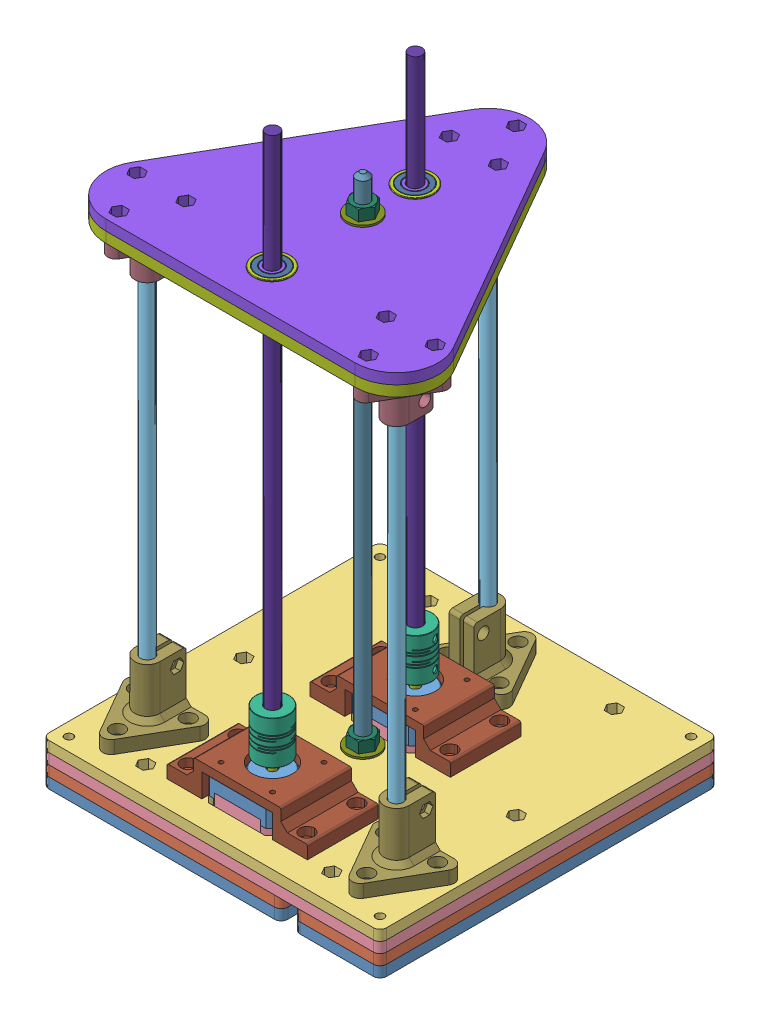
SolidWorks assembly 02_00_Assy_z_axis_V1, configuration Défaut. Lengths in mm.
Overall size (203.2 380.91 203.2).
110 component instances, 54 part files, 69 mates.
Components (placement in the parent):
- 02_01_Assy_base_z_axis_V1-1: 02_01_Assy_base_z_axis_V1 [Défaut] at (-233.6469 0 294.9138) size (203.2 25.4 203.2)
  - 02_03_plaque_fond_base-1: 02_03_plaque_fond_base [Défaut] at (80.101 0 119.7934) size (203.2 6.35 203.2)
  - 02_05_deuxieme_niveau_base-1: 02_05_deuxieme_niveau_base [Défaut] at (80.101 6.35 119.7934) x (-1 0 0) z (0 0 -1) size (203.2 6.35 203.2)
  - 02_06_troixieme_niveau_base-1: 02_06_troixieme_niveau_base [Défaut] at (80.101 19.05 119.7934) x (-1 0 0) z (0 0 -1) size (203.2 6.35 203.2)
  - 02_012_deuxieme_v2_niveau_base-1: 02_012_deuxieme_v2_niveau_base [Défaut] at (80.101 12.7 119.7934) x (-1 0 0) z (0 0 -1) size (203.2 6.35 203.2)
- Stainless_Steel_Rod_8_290-1: Stainless_Steel_Rod_8_290 [1274T471] at (-228.5459 151.35 479.7071) x (0.927753 0 -0.373195) z (0 -1 0) size (8 8 290)
- Stainless_Steel_Rod_8_290-2: Stainless_Steel_Rod_8_290 [1274T471] at (-78.5444 151.35 479.7063) x (-0.988682 0 -0.150024) z (0 -1 0) size (8 8 290)
- Stainless_Steel_Rod_8_290-3: Stainless_Steel_Rod_8_290 [1274T471] at (-153.5459 151.35 349.7071) x (-0.878649 0 -0.477467) z (0 1 0) size (8 8 290)
- NEMA17_Coupler-1: NEMA17_Coupler [Default] at (-153.3959 48.5 479.5571) x (-0.967472 0 -0.252977) z (0.252977 0 -0.967472) size (26.77 26 23.11)
- 02_09_support_trois_rods_haut-1: 02_09_support_trois_rods_haut [Défaut] at (-153.5451 290 414.7071) x (-1 0 0.000011) z (-0.000011 0 -1) size (200 6.35 180)
- 02_10_support_haut-1: 02_10_support_haut [Défaut] at (-153.5451 296.35 414.7071) x (-1 0 0.000011) z (-0.000011 0 -1) size (200 6.35 180)
- 608-2RS Skate Board Ball Bearing.step-2: 608-2RS Skate Board Ball Bearing.step [Défaut] at (-153.5444 299.85 479.7071) x (0 -1 0) z (0 0 1) size (7 22 22)
  - Ball 001.step-1: Ball 001.step [Défaut] at origin size (4 4 4)
  - Ball 002.step-1: Ball 002.step [Défaut] x (1 0 0) z (0 0.781831 0.62349) size (4 4 4)
  - Ball 003.step-1: Ball 003.step [Défaut] x (1 0 0) z (0 0.974928 -0.222521) size (4 4 4)
  - Ball 004.step-1: Ball 004.step [Défaut] x (1 0 0) z (0 0.433884 -0.900969) size (4 4 4)
  - Ball 005.step-1: Ball 005.step [Défaut] x (1 0 0) z (0 -0.433884 -0.900969) size (4 4 4)
  - Ball 006.step-1: Ball 006.step [Défaut] x (1 0 0) z (0 -0.974928 -0.222521) size (4 4 4)
  - Ball 007.step-1: Ball 007.step [Défaut] x (1 0 0) z (0 -0.781831 0.62349) size (4 4 4)
  - Cage 001.step-1: Cage 001.step [Défaut] x (1 0 0) z (0 1 0) size (2.12 17 16.8)
  - Cage 002.step-1: Cage 002.step [Défaut] x (-1 0 0) z (0 0 -1) size (2.12 16.8 17)
  - Rivet 002.step-1: Rivet 002.step [Défaut] x (1 0 0) z (0 -0.781831 0.62349) size (0.42 0.6 0.6)
  - Rivet 003.step-1: Rivet 003.step [Défaut] x (1 0 0) z (0 -0.974928 -0.222521) size (0.42 0.6 0.6)
  - Rivet 001.step-1: Rivet 001.step [Défaut] x (1 0 0) z (0 -0.433884 0.900969) size (0.42 0.6 0.6)
  - Rivet 004.step-1: Rivet 004.step [Défaut] x (1 0 0) z (0 -0.433884 -0.900969) size (0.42 0.6 0.6)
  - Rivet 005.step-1: Rivet 005.step [Défaut] x (1 0 0) z (0 0.433884 -0.900969) size (0.42 0.6 0.6)
  - Rivet 006.step-1: Rivet 006.step [Défaut] x (1 0 0) z (0 0.974928 -0.222521) size (0.42 0.6 0.6)
  - Rivet 007.step-1: Rivet 007.step [Défaut] x (1 0 0) z (0 0.781831 0.62349) size (0.42 0.6 0.6)
  - Outer Ring001.step-1: Outer Ring001.step [Défaut] at origin size (7 22 22)
  - Inner Ring001.step-1: Inner Ring001.step [Défaut] at origin size (7 12 12)
  - Seal 001.step-1: Seal 001.step [Défaut] at origin size (0.6 19 19)
  - Seal 002.step-1: Seal 002.step [Défaut] x (-1 0 0) z (0 0 -1) size (0.6 19 19)
- 02_11_support_moteur-1: 02_11_support_moteur [Défaut] at (-153.3959 39.5 479.5571) size (84.5 19.1 42.5)
- 02_13_support_rodes_8mm_base-1: 02_13_support_rodes_8mm_base [Défaut] at (-78.5444 25.4 479.7063) x (-1 0 0) z (0 0 -1) size (47.68 37.8 42.63)
- 02_13_support_rodes_8mm_base-2: 02_13_support_rodes_8mm_base [Défaut] at (-228.5459 25.4 479.7071) x (-1 0 0) z (0 0 -1) size (47.68 37.8 42.63)
- 02_13_support_rodes_8mm_base-3: 02_13_support_rodes_8mm_base [Défaut] at (-153.5459 25.4 349.7071) size (47.68 37.8 42.63)
- 02_14_support_rodes_8mm_haut-1: 02_14_support_rodes_8mm_haut [Défaut] at (-78.5444 290 479.7063) x (1 0 -0.000011) z (-0.000011 0 -1) size (42.68 27.8 38.3)
- 02_14_support_rodes_8mm_haut-2: 02_14_support_rodes_8mm_haut [Défaut] at (-228.5459 290 479.7071) x (1 0 -0.000011) z (-0.000011 0 -1) size (42.68 27.8 38.3)
- 02_14_support_rodes_8mm_haut-3: 02_14_support_rodes_8mm_haut [Défaut] at (-153.5459 290 349.7071) x (-1 0 0.000011) z (0.000011 0 1) size (42.68 27.8 38.3)
- Lead Screw_M12-1: Lead Screw_M12 [97048A742] at (-153.5459 162.5 425.0321) x (-0.414721 0 0.909949) z (0 -1 0) size (7.9 7.9 325)
- 95462A510_Medium-Strength Steel Hex Nut-2: 95462A510_Medium-Strength Steel Hex Nut [95462A510] at (-153.5459 307.1656 425.0321) x (0.86602 0 -0.50001) z (0 1 0) size (12.7 14.66 6.75)
- 516_washer-1: 516_washer [90107A030] at (-153.5459 302.7 425.0321) size (19.05 1.09 19.05)
- 516_washer-2: 516_washer [90107A030] at (-153.5459 25.4 425.0321) size (19.05 1.09 19.05)
- T8_lead_screw_300mm-1: T8_lead_screw_300mm [1274T471] at (-153.3959 223.9115 479.5571) x (0.654232 0 0.756294) z (0 1 0) size (8 8 300)
- 02_11_support_moteur-2: 02_11_support_moteur [Défaut] at (-153.3959 39.5 393.5571) size (84.5 19.1 42.5)
- 95462A510_Medium-Strength Steel Hex Nut-4: 95462A510_Medium-Strength Steel Hex Nut [95462A510] at (-153.5459 29.8656 425.0321) x (0.866025 0 -0.5) z (0 1 0) size (12.7 14.66 6.75)
- 608-2RS Skate Board Ball Bearing.step-3: 608-2RS Skate Board Ball Bearing.step [Défaut] at (-153.5454 299.85 393.7071) x (0 -1 0) z (0.672808 0 0.739817) size (7 22 22)
  - Ball 001.step-1: Ball 001.step [Défaut] at origin size (4 4 4)
  - Ball 002.step-1: Ball 002.step [Défaut] x (1 0 0) z (0 0.781831 0.62349) size (4 4 4)
  - Ball 003.step-1: Ball 003.step [Défaut] x (1 0 0) z (0 0.974928 -0.222521) size (4 4 4)
  - Ball 004.step-1: Ball 004.step [Défaut] x (1 0 0) z (0 0.433884 -0.900969) size (4 4 4)
  - Ball 005.step-1: Ball 005.step [Défaut] x (1 0 0) z (0 -0.433884 -0.900969) size (4 4 4)
  - Ball 006.step-1: Ball 006.step [Défaut] x (1 0 0) z (0 -0.974928 -0.222521) size (4 4 4)
  - Ball 007.step-1: Ball 007.step [Défaut] x (1 0 0) z (0 -0.781831 0.62349) size (4 4 4)
  - Cage 001.step-1: Cage 001.step [Défaut] x (1 0 0) z (0 1 0) size (2.12 17 16.8)
  - Cage 002.step-1: Cage 002.step [Défaut] x (-1 0 0) z (0 0 -1) size (2.12 16.8 17)
  - Rivet 002.step-1: Rivet 002.step [Défaut] x (1 0 0) z (0 -0.781831 0.62349) size (0.42 0.6 0.6)
  - Rivet 003.step-1: Rivet 003.step [Défaut] x (1 0 0) z (0 -0.974928 -0.222521) size (0.42 0.6 0.6)
  - Rivet 001.step-1: Rivet 001.step [Défaut] x (1 0 0) z (0 -0.433884 0.900969) size (0.42 0.6 0.6)
  - Rivet 004.step-1: Rivet 004.step [Défaut] x (1 0 0) z (0 -0.433884 -0.900969) size (0.42 0.6 0.6)
  - Rivet 005.step-1: Rivet 005.step [Défaut] x (1 0 0) z (0 0.433884 -0.900969) size (0.42 0.6 0.6)
  - Rivet 006.step-1: Rivet 006.step [Défaut] x (1 0 0) z (0 0.974928 -0.222521) size (0.42 0.6 0.6)
  - Rivet 007.step-1: Rivet 007.step [Défaut] x (1 0 0) z (0 0.781831 0.62349) size (0.42 0.6 0.6)
  - Outer Ring001.step-1: Outer Ring001.step [Défaut] at origin size (7 22 22)
  - Inner Ring001.step-1: Inner Ring001.step [Défaut] at origin size (7 12 12)
  - Seal 001.step-1: Seal 001.step [Défaut] at origin size (0.6 19 19)
  - Seal 002.step-1: Seal 002.step [Défaut] x (-1 0 0) z (0 0 -1) size (0.6 19 19)
- NEMA17_Coupler-2: NEMA17_Coupler [Default] at (-153.3959 48.5 393.5571) x (-0.262561 0 -0.964915) z (0.964915 0 -0.262561) size (26.77 26 23.11)
- T8_lead_screw_300mm-2: T8_lead_screw_300mm [1274T471] at (-153.3959 222 393.5571) x (0.996676 0 0.081473) z (0 -1 0) size (8 8 300)
- 95462A510_Medium-Strength Steel Hex Nut-5: 95462A510_Medium-Strength Steel Hex Nut [95462A510] at (-153.5459 3.3734 425.0321) x (0.866025 0 -0.5) z (0 -1 0) size (12.7 14.66 6.75)
- NEMA17 x 33.step-1: NEMA17 x 33.step [Défaut] at (-153.3959 39.5 393.5571) x (0 0 1) z (1 0 0) size (42 70.5 60)
  - Copper-2of4.step-1: Copper-2of4.step [Défaut] at (0 28 0) x (0 1 0) z (0 0 1) size (2.77 3.05 24)
  - Frontplate.step-1: Frontplate.step [Défaut] at (0 10.5 0) size (42 12.5 42)
  - Backplate.step-1: Backplate.step [Défaut] at (0 33 0) size (42 10.5 42)
  - Connenctor.step-1: Connenctor.step [Défaut] at (0 24.5 22) size (7 7 7)
  - Housing.step-1: Housing.step [Défaut] at (0 7.5 0) size (42 32 42)
  - Bearing dummy.step-1: Bearing dummy.step [Défaut] at (0 4 0) size (22 7 22)
  - Bearing dummy 01.step-1: Bearing dummy 01.step [Défaut] at (0 28 0) size (22 7 22)
  - Core.step-1: Core.step [Défaut] at origin size (30 70.5 30)
  - M3x25-Screw.step-1: M3x25-Screw.step [Défaut] at (15.5 30.6 15.5) x (1 0 0) z (0 1 0) size (5.5 5.5 27)
  - M3x25-Screw004.step-1: M3x25-Screw004.step [Défaut] at (-15.5 30.6 15.5) x (1 0 0) z (0 1 0) size (5.5 5.5 27)
  - M3x25-Screw005.step-1: M3x25-Screw005.step [Défaut] at (-15.5 30.6 -15.5) x (1 0 0) z (0 1 0) size (5.5 5.5 27)
  - M3x25-Screw006.step-1: M3x25-Screw006.step [Défaut] at (15.5 30.6 -15.5) x (1 0 0) z (0 1 0) size (5.5 5.5 27)
  - Cable-1of4.step-1: Cable-1of4.step [Défaut] at (0 28 0) size (3.44 3.69 21)
  - Copper-1of4.step-1: Copper-1of4.step [Défaut] at (0 28 0) size (2.77 3.05 24)
  - Cable-2of4.step-1: Cable-2of4.step [Défaut] at (0 28 0) x (0 1 0) z (0 0 1) size (3.44 3.69 21)
  - Copper-4of4.step-1: Copper-4of4.step [Défaut] at (0 28 0) x (0 -1 0) z (0 0 1) size (2.77 3.05 24)
  - Cable-3of4.step-1: Cable-3of4.step [Défaut] at (0 28 0) x (-1 0 0) z (0 0 1) size (3.44 3.69 21)
  - Copper-3of4.step-1: Copper-3of4.step [Défaut] at (0 28 0) x (-1 0 0) z (0 0 1) size (2.77 3.05 24)
  - Cable-4of4.step-1: Cable-4of4.step [Défaut] at (0 28 0) x (0 -1 0) z (0 0 1) size (3.44 3.69 21)
- NEMA17 x 33.step-2: NEMA17 x 33.step [Défaut] at (-153.3959 39.5 479.5571) x (0 0 1) z (1 0 0) size (42 70.5 60)
  - Copper-2of4.step-1: Copper-2of4.step [Défaut] at (0 28 0) x (0 1 0) z (0 0 1) size (2.77 3.05 24)
  - Frontplate.step-1: Frontplate.step [Défaut] at (0 10.5 0) size (42 12.5 42)
  - Backplate.step-1: Backplate.step [Défaut] at (0 33 0) size (42 10.5 42)
  - Connenctor.step-1: Connenctor.step [Défaut] at (0 24.5 22) size (7 7 7)
  - Housing.step-1: Housing.step [Défaut] at (0 7.5 0) size (42 32 42)
  - Bearing dummy.step-1: Bearing dummy.step [Défaut] at (0 4 0) size (22 7 22)
  - Bearing dummy 01.step-1: Bearing dummy 01.step [Défaut] at (0 28 0) size (22 7 22)
  - Core.step-1: Core.step [Défaut] at origin size (30 70.5 30)
  - M3x25-Screw.step-1: M3x25-Screw.step [Défaut] at (15.5 30.6 15.5) x (1 0 0) z (0 1 0) size (5.5 5.5 27)
  - M3x25-Screw004.step-1: M3x25-Screw004.step [Défaut] at (-15.5 30.6 15.5) x (1 0 0) z (0 1 0) size (5.5 5.5 27)
  - M3x25-Screw005.step-1: M3x25-Screw005.step [Défaut] at (-15.5 30.6 -15.5) x (1 0 0) z (0 1 0) size (5.5 5.5 27)
  - M3x25-Screw006.step-1: M3x25-Screw006.step [Défaut] at (15.5 30.6 -15.5) x (1 0 0) z (0 1 0) size (5.5 5.5 27)
  - Cable-1of4.step-1: Cable-1of4.step [Défaut] at (0 28 0) size (3.44 3.69 21)
  - Copper-1of4.step-1: Copper-1of4.step [Défaut] at (0 28 0) size (2.77 3.05 24)
  - Cable-2of4.step-1: Cable-2of4.step [Défaut] at (0 28 0) x (0 1 0) z (0 0 1) size (3.44 3.69 21)
  - Copper-4of4.step-1: Copper-4of4.step [Défaut] at (0 28 0) x (0 -1 0) z (0 0 1) size (2.77 3.05 24)
  - Cable-3of4.step-1: Cable-3of4.step [Défaut] at (0 28 0) x (-1 0 0) z (0 0 1) size (3.44 3.69 21)
  - Copper-3of4.step-1: Copper-3of4.step [Défaut] at (0 28 0) x (-1 0 0) z (0 0 1) size (2.77 3.05 24)
  - Cable-4of4.step-1: Cable-4of4.step [Défaut] at (0 28 0) x (0 -1 0) z (0 0 1) size (3.44 3.69 21)
Mates (geometry in assembly coordinates):
- Coïncidente1: coincident anti-aligned: plane of 02_01_Assy_base_z_axis_V1-1/02_03_plaque_fond_base-1 through (-153.5459 0 414.7071) normal (0 -1 0)
- Coïncidente4: coincident anti-aligned: plane of 02_01_Assy_base_z_axis_V1-1/02_03_plaque_fond_base-1 through (-153.5459 6.35 414.7071) normal (0 1 0); plane of Stainless_Steel_Rod_8_290-1 through (-228.5459 6.35 479.7071) normal (0 -1 0)
- Coïncidente5: coincident anti-aligned: plane of 02_01_Assy_base_z_axis_V1-1/02_03_plaque_fond_base-1 through (-153.5459 6.35 414.7071) normal (0 1 0); plane of Stainless_Steel_Rod_8_290-2 through (-78.5444 6.35 479.7063) normal (0 -1 0)
- Coïncidente6: coincident anti-aligned: plane of 02_01_Assy_base_z_axis_V1-1/02_03_plaque_fond_base-1 through (-153.5459 6.35 414.7071) normal (0 1 0); plane of Stainless_Steel_Rod_8_290-3 through (-153.5459 6.35 349.7071) normal (0 -1 0)
- Coïncidente29: coincident aligned: plane of Stainless_Steel_Rod_8_290-1 through (-228.5459 296.35 479.7071) normal (0 1 0); plane of 02_09_support_trois_rods_haut-1 through (-78.5444 296.35 479.7063) normal (0 1 0)
- Coaxiale20: concentric aligned: cylinder of Stainless_Steel_Rod_8_290-3 through (-153.5459 296.35 349.7071) axis (0 -1 0) radius 4; cylinder of 02_09_support_trois_rods_haut-1 through (-153.5459 296.35 349.7071) axis (0 -1 0) radius 3.925
- Coaxiale21: concentric anti-aligned: cylinder of Stainless_Steel_Rod_8_290-2 through (-78.5444 6.35 479.7063) axis (0 1 0) radius 4; cylinder of 02_09_support_trois_rods_haut-1 through (-78.5444 296.35 479.7063) axis (0 -1 0) radius 3.925
- Coïncidente30: coincident anti-aligned: plane of 02_09_support_trois_rods_haut-1 through (-78.5444 296.35 479.7063) normal (0 1 0); plane of 02_10_support_haut-1 through (-78.5444 296.35 479.7063) normal (0 -1 0)
- Coaxiale22: concentric aligned: cylinder of 02_09_support_trois_rods_haut-1 through (-153.5444 296.35 479.7071) axis (0 -1 0) radius 5.7; cylinder of 02_10_support_haut-1 through (-153.5444 302.7 479.7071) axis (0 -1 0) radius 11
- Coïncidente31: coincident aligned: plane of 02_09_support_trois_rods_haut-1 through (-56.8899 296.35 467.213) normal (0.86618 0 -0.499732); plane of 02_10_support_haut-1 through (-56.8899 302.7 467.213) normal (0.86618 0 -0.499732)
- Coïncidente32: coincident anti-aligned: plane of 02_09_support_trois_rods_haut-1 through (-78.5444 296.35 479.7063) normal (0 1 0); plane of 608-2RS Skate Board Ball Bearing.step-2/Inner Ring001.step-1 through (-153.5444 296.35 479.7071) normal (0 -1 0)
- Coaxiale23: concentric anti-aligned: cylinder of 02_09_support_trois_rods_haut-1 through (-153.5444 296.35 479.7071) axis (0 -1 0) radius 5.7; cylinder of 608-2RS Skate Board Ball Bearing.step-2/Inner Ring001.step-1 through (-153.5444 296.35 479.7071) axis (0 1 0) radius 4
- Coaxiale26: concentric aligned: cylinder of Stainless_Steel_Rod_8_290-2 through (-78.5444 6.35 479.7063) axis (0 1 0) radius 4; cylinder of 02_13_support_rodes_8mm_base-1 through (-78.5444 25.4 479.7063) axis (0 1 0) radius 4.075
- Coïncidente36: coincident anti-aligned: plane of 02_01_Assy_base_z_axis_V1-1/02_06_troixieme_niveau_base-1 through (-153.5459 25.4 414.7071) normal (0 1 0); plane of 02_13_support_rodes_8mm_base-1 through (-78.5444 25.4 479.7063) normal (0 -1 0)
- Coaxiale27: concentric anti-aligned: cylinder of Stainless_Steel_Rod_8_290-3 through (-153.5459 296.35 349.7071) axis (0 -1 0) radius 4; cylinder of 02_13_support_rodes_8mm_base-3 through (-153.5459 25.4 349.7071) axis (0 1 0) radius 4.075
- Coïncidente38: coincident anti-aligned: plane of 02_01_Assy_base_z_axis_V1-1/02_06_troixieme_niveau_base-1 through (-153.5459 25.4 414.7071) normal (0 1 0); plane of 02_13_support_rodes_8mm_base-3 through (-153.5459 25.4 349.7071) normal (0 -1 0)
- Parallèle3: parallel anti-aligned: plane of 02_01_Assy_base_z_axis_V1-1/02_06_troixieme_niveau_base-1 through (-51.9459 25.4 516.3071) normal (0 0 1); plane of 02_13_support_rodes_8mm_base-1 through (-51.0444 33.2 463.8292) normal (0 0 -1)
- Coïncidente41: coincident anti-aligned: plane of 02_01_Assy_base_z_axis_V1-1/02_06_troixieme_niveau_base-1 through (-153.5459 25.4 414.7071) normal (0 1 0); plane of 02_13_support_rodes_8mm_base-2 through (-228.5459 25.4 479.7071) normal (0 -1 0)
- Coaxiale28: concentric aligned: cylinder of Stainless_Steel_Rod_8_290-1 through (-228.5459 6.35 479.7071) axis (0 1 0) radius 4; cylinder of 02_13_support_rodes_8mm_base-2 through (-228.5459 25.4 479.7071) axis (0 1 0) radius 4.075
- Parallèle4: parallel anti-aligned: plane of 02_01_Assy_base_z_axis_V1-1/02_06_troixieme_niveau_base-1 through (-51.9459 25.4 516.3071) normal (0 0 1); plane of 02_13_support_rodes_8mm_base-2 through (-201.0459 33.2 463.83) normal (0 0 -1)
- Coïncidente46: coincident anti-aligned: plane of 02_09_support_trois_rods_haut-1 through (-78.5444 290 479.7063) normal (0 -1 0); plane of 02_14_support_rodes_8mm_haut-2 through (-228.5459 290 479.7071) normal (0 1 0)
- Coaxiale30: concentric anti-aligned: cylinder of Stainless_Steel_Rod_8_290-1 through (-228.5459 6.35 479.7071) axis (0 1 0) radius 4; cylinder of 02_14_support_rodes_8mm_haut-2 through (-228.5459 290 479.7071) axis (0 -1 0) radius 4.075
- Parallèle5: parallel anti-aligned: plane of 02_09_support_trois_rods_haut-1 through (-78.5441 296.35 504.7063) normal (0.000011 0 1); plane of 02_14_support_rodes_8mm_haut-2 through (-253.546 282.2 465.2737) normal (-0.000011 0 -1)
- Coïncidente48: coincident anti-aligned: plane of 02_09_support_trois_rods_haut-1 through (-78.5444 290 479.7063) normal (0 -1 0); plane of 02_14_support_rodes_8mm_haut-1 through (-78.5444 290 479.7063) normal (0 1 0)
- Coaxiale31: concentric anti-aligned: cylinder of 02_14_support_rodes_8mm_haut-1 through (-78.5444 290 479.7063) axis (0 -1 0) radius 4.075; cylinder of Stainless_Steel_Rod_8_290-2 through (-78.5444 6.35 479.7063) axis (0 1 0) radius 4
- Parallèle7: parallel anti-aligned: plane of 02_09_support_trois_rods_haut-1 through (-78.5441 296.35 504.7063) normal (0.000011 0 1); plane of 02_14_support_rodes_8mm_haut-1 through (-103.5446 282.2 465.2728) normal (-0.000011 0 -1)
- Coïncidente51: coincident anti-aligned: plane of 02_09_support_trois_rods_haut-1 through (-78.5444 290 479.7063) normal (0 -1 0); plane of 02_14_support_rodes_8mm_haut-3 through (-153.5459 290 349.7071) normal (0 1 0)
- Coaxiale32: concentric aligned: cylinder of Stainless_Steel_Rod_8_290-3 through (-153.5459 296.35 349.7071) axis (0 -1 0) radius 4; cylinder of 02_14_support_rodes_8mm_haut-3 through (-153.5459 290 349.7071) axis (0 -1 0) radius 4.075
- Coaxiale34: concentric anti-aligned: cylinder of 02_10_support_haut-1 through (-153.5459 296.35 425.0321) axis (0 1 0) radius 4; cylinder of Lead Screw_M12-1 through (-153.5459 0 425.0321) axis (0 -1 0) radius 3.95
- Coïncidente52: coincident aligned: plane of 02_01_Assy_base_z_axis_V1-1/02_03_plaque_fond_base-1 through (-153.5459 0 414.7071) normal (0 -1 0); plane of Lead Screw_M12-1 through (-157.1402 0 423.394) normal (0 -1 0)
- Coaxiale38: concentric anti-aligned: cylinder of 02_01_Assy_base_z_axis_V1-1/02_06_troixieme_niveau_base-1 through (-153.5459 19.05 349.7071) axis (0 1 0) radius 3.925; cylinder of Stainless_Steel_Rod_8_290-3 through (-153.5459 296.35 349.7071) axis (0 -1 0) radius 4
- Parallèle13: parallel anti-aligned: plane of 02_01_Assy_base_z_axis_V1-1/02_03_plaque_fond_base-1 through (-255.1459 6.35 313.1071) normal (0 0 -1); plane of 02_13_support_rodes_8mm_base-3 through (-181.0459 33.2 365.5843) normal (0 0 1)
- Parallèle14: parallel aligned: plane of 02_09_support_trois_rods_haut-1 through (-78.5441 296.35 504.7063) normal (0.000011 0 1); plane of 02_14_support_rodes_8mm_haut-3 through (-128.5457 282.2 364.1406) normal (0.000011 0 1)
- Coaxiale43: concentric aligned: cylinder of 02_01_Assy_base_z_axis_V1-1/02_06_troixieme_niveau_base-1 through (-228.5459 19.05 479.7071) axis (0 1 0) radius 3.925; cylinder of Stainless_Steel_Rod_8_290-1 through (-228.5459 6.35 479.7071) axis (0 1 0) radius 4
- Parallèle15: parallel anti-aligned: plane of 02_01_Assy_base_z_axis_V1-1/02_06_troixieme_niveau_base-1 through (-51.9459 25.4 516.3071) normal (0 0 1); plane of 02_13_support_rodes_8mm_base-2 through (-201.0459 33.2 463.83) normal (0 0 -1)
- Coaxiale48: concentric aligned: cylinder of Lead Screw_M12-1 through (-153.5459 0 425.0321) axis (0 -1 0) radius 3.95; cylinder of 95462A510_Medium-Strength Steel Hex Nut-2 through (-153.5459 310.5391 425.0321) axis (0 -1 0) radius 3.9688
- Coaxiale49: concentric anti-aligned: cylinder of Lead Screw_M12-1 through (-153.5459 0 425.0321) axis (0 -1 0) radius 3.95; cylinder of 516_washer-1 through (-153.5459 302.7 425.0321) axis (0 1 0) radius 4.3688
- Coïncidente69: coincident anti-aligned: plane of 02_10_support_haut-1 through (-78.5444 302.7 479.7063) normal (0 1 0); plane of 516_washer-1 through (-153.5459 302.7 425.0321) normal (0 -1 0)
- Coïncidente70: coincident anti-aligned: plane of 95462A510_Medium-Strength Steel Hex Nut-2 through (-160.8782 303.7922 425.0322) normal (0 -1 0); plane of 516_washer-1 through (-153.5459 303.7922 425.0321) normal (0 1 0)
- Parallèle19: parallel aligned: plane of 02_10_support_haut-1 through (-78.5441 302.7 504.7063) normal (0.000011 0 1); plane of 95462A510_Medium-Strength Steel Hex Nut-2 through (-157.212 310.5391 431.3822) normal (0.000011 0 1)
- Coïncidente72: coincident anti-aligned: plane of 02_01_Assy_base_z_axis_V1-1/02_06_troixieme_niveau_base-1 through (-153.5459 25.4 414.7071) normal (0 1 0); plane of 516_washer-2 through (-153.5459 25.4 425.0321) normal (0 -1 0)
- Coaxiale53: concentric aligned: cylinder of NEMA17_Coupler-1 through (-153.3959 48.5 479.5571) axis (0 -1 0) radius 4.025; cylinder of T8_lead_screw_300mm-1 through (-153.3959 373.9115 479.5571) axis (0 -1 0) radius 4
- Coaxiale58: concentric aligned: cylinder of 02_01_Assy_base_z_axis_V1-1/02_06_troixieme_niveau_base-1 through (-153.5459 19.05 425.0321) axis (0 1 0) radius 4; cylinder of 516_washer-2 through (-153.5459 25.4 425.0321) axis (0 1 0) radius 4.3688
- Coïncidente84: coincident: plane of 02_11_support_moteur-1 through (-179.6459 39.5 479.5571) normal (-1 0 0); plane of 02_11_support_moteur-2 through (-179.6459 61.288 393.5571) normal (-1 0 0)
- Coaxiale61: concentric anti-aligned: cylinder of Lead Screw_M12-1 through (-153.5459 0 425.0321) axis (0 -1 0) radius 3.95; circle of 95462A510_Medium-Strength Steel Hex Nut-4
- Coïncidente89: coincident anti-aligned: plane of 516_washer-2 through (-153.5459 26.4922 425.0321) normal (0 1 0); plane of 95462A510_Medium-Strength Steel Hex Nut-4 through (-160.8782 26.4922 425.0321) normal (0 -1 0)
- Parallèle25: parallel aligned: plane of 02_01_Assy_base_z_axis_V1-1/02_06_troixieme_niveau_base-1 through (-51.9459 25.4 516.3071) normal (0 0 1); plane of 95462A510_Medium-Strength Steel Hex Nut-4 through (-157.2121 33.2391 431.3821) normal (0 0 1)
- Coaxiale62: concentric anti-aligned: cylinder of 02_10_support_haut-1 through (-153.5454 296.35 393.7071) axis (0 1 0) radius 11; cylinder of 608-2RS Skate Board Ball Bearing.step-3/Outer Ring001.step-1 through (-153.5454 303.35 393.7071) axis (0 -1 0) radius 11
- Coïncidente91: coincident anti-aligned: plane of 02_09_support_trois_rods_haut-1 through (-78.5444 296.35 479.7063) normal (0 1 0); plane of 608-2RS Skate Board Ball Bearing.step-3/Outer Ring001.step-1 through (-153.5454 296.35 393.7071) normal (0 -1 0)
- Coaxiale64: concentric anti-aligned: cylinder of NEMA17_Coupler-2 through (-153.3959 48.5 393.5571) axis (0 -1 0) radius 4.025; cylinder of T8_lead_screw_300mm-2 through (-153.3959 72 393.5571) axis (0 1 0) radius 4
- Coaxiale65: concentric anti-aligned: cylinder of Lead Screw_M12-1 through (-153.5459 0 425.0321) axis (0 -1 0) radius 3.95; cylinder of 95462A510_Medium-Strength Steel Hex Nut-5 through (-153.5459 0 425.0321) axis (0 1 0) radius 3.9688
- Coaxiale66: concentric anti-aligned: cylinder of 02_01_Assy_base_z_axis_V1-1/02_012_deuxieme_v2_niveau_base-1 through (-153.5459 12.7 425.0321) axis (0 1 0) radius 4; cylinder of Lead Screw_M12-1 through (-153.5459 0 425.0321) axis (0 -1 0) radius 3.95
- Parallèle26: parallel aligned: plane of 02_01_Assy_base_z_axis_V1-1/02_03_plaque_fond_base-1 through (-157.1976 0 418.7071) normal (0.866025 0 0.5); plane of 95462A510_Medium-Strength Steel Hex Nut-5 through (-146.2135 0 425.0321) normal (0.866025 0 0.5)
- Coïncidente95: coincident aligned: plane of 02_01_Assy_base_z_axis_V1-1/02_03_plaque_fond_base-1 through (-153.5459 0 414.7071) normal (0 -1 0); plane of 95462A510_Medium-Strength Steel Hex Nut-5 through (-157.2121 0 431.3821) normal (0 -1 0)
- Coïncidente97: coincident aligned: plane of 02_01_Assy_base_z_axis_V1-1/02_03_plaque_fond_base-1 through (-153.5459 0 414.7071) normal (0 -1 0); plane of NEMA17 x 33.step-2/Housing.step-1 through (-153.3959 0 479.5571) normal (0 -1 0)
- Coïncidente98: coincident aligned: plane of 02_01_Assy_base_z_axis_V1-1/02_03_plaque_fond_base-1 through (-153.5459 0 414.7071) normal (0 -1 0); plane of NEMA17 x 33.step-1/Housing.step-1 through (-153.3959 0 393.5571) normal (0 -1 0)
- Coïncidente99: coincident anti-aligned: plane of 02_01_Assy_base_z_axis_V1-1/02_03_plaque_fond_base-1 through (-132.3959 0 462.7291) normal (-1 0 0); plane of NEMA17 x 33.step-2/Housing.step-1 through (-132.3959 32 465.718) normal (1 0 0)
- Coïncidente100: coincident anti-aligned: plane of 02_01_Assy_base_z_axis_V1-1/02_06_troixieme_niveau_base-1 through (-136.5678 19.05 458.5571) normal (0 0 1); plane of NEMA17 x 33.step-2/Frontplate.step-1 through (-136.4253 29 458.5571) normal (0 0 -1)
- Coïncidente101: coincident anti-aligned: plane of 02_01_Assy_base_z_axis_V1-1/02_06_troixieme_niveau_base-1 through (-132.3959 19.05 376.7291) normal (-1 0 0); plane of NEMA17 x 33.step-1/Frontplate.step-1 through (-132.3959 29 410.5277) normal (1 0 0)
- Coïncidente102: coincident anti-aligned: plane of 02_01_Assy_base_z_axis_V1-1/02_06_troixieme_niveau_base-1 through (-170.5239 19.05 372.5571) normal (0 0 1); plane of NEMA17 x 33.step-1/Frontplate.step-1 through (-136.4253 29 372.5571) normal (0 0 -1)
- Coïncidente103: coincident anti-aligned: plane of NEMA17_Coupler-1 through (-156.0758 48.5 478.8564) normal (0 -1 0); plane of NEMA17 x 33.step-2/Core.step-1 through (-151.1459 48.5 479.5571) normal (0 1 0)
- Coaxiale69: concentric aligned: circle of NEMA17_Coupler-1; cylinder of NEMA17 x 33.step-2/Core.step-1 through (-153.3959 63.2 479.5571) axis (0 -1 0) radius 2.5
- Coïncidente104: coincident anti-aligned: plane of NEMA17_Coupler-2 through (-154.1232 48.5 390.8843) normal (0 -1 0); plane of NEMA17 x 33.step-1/Core.step-1 through (-151.1459 48.5 393.5571) normal (0 1 0)
- Coaxiale70: concentric aligned: circle of NEMA17_Coupler-2; cylinder of NEMA17 x 33.step-1/Core.step-1 through (-153.3959 63.2 393.5571) axis (0 -1 0) radius 2.5
- Coaxiale73: concentric anti-aligned: cylinder of 02_11_support_moteur-1 through (-168.8959 39.5 495.0571) axis (0 1 0) radius 1.325; cylinder of NEMA17 x 33.step-2/Frontplate.step-1 through (-168.8959 29 495.0571) axis (0 -1 0) radius 1.23
- Coaxiale74: concentric anti-aligned: cylinder of 02_11_support_moteur-1 through (-137.8959 39.5 464.0571) axis (0 1 0) radius 1.325; cylinder of NEMA17 x 33.step-2/Frontplate.step-1 through (-137.8959 29 464.0571) axis (0 -1 0) radius 1.23
- Coïncidente106: coincident anti-aligned: plane of 02_11_support_moteur-1 through (-153.3959 39.5 479.5571) normal (0 -1 0); plane of NEMA17 x 33.step-2/Frontplate.step-1 through (-153.3959 39.5 479.5571) normal (0 1 0)
- Coaxiale75: concentric: cylinder of 02_11_support_moteur-2 through (-137.8959 61.288 409.0571) axis (0 1 0) radius 1.325; cylinder of NEMA17 x 33.step-1/Frontplate.step-1 through (-137.8959 29 409.0571) axis (0 -1 0) radius 1.23
- Coïncidente107: coincident anti-aligned: plane of 02_11_support_moteur-2 through (-153.3959 39.5 393.5571) normal (0 -1 0); plane of NEMA17 x 33.step-1/Frontplate.step-1 through (-153.3959 39.5 393.5571) normal (0 1 0)
